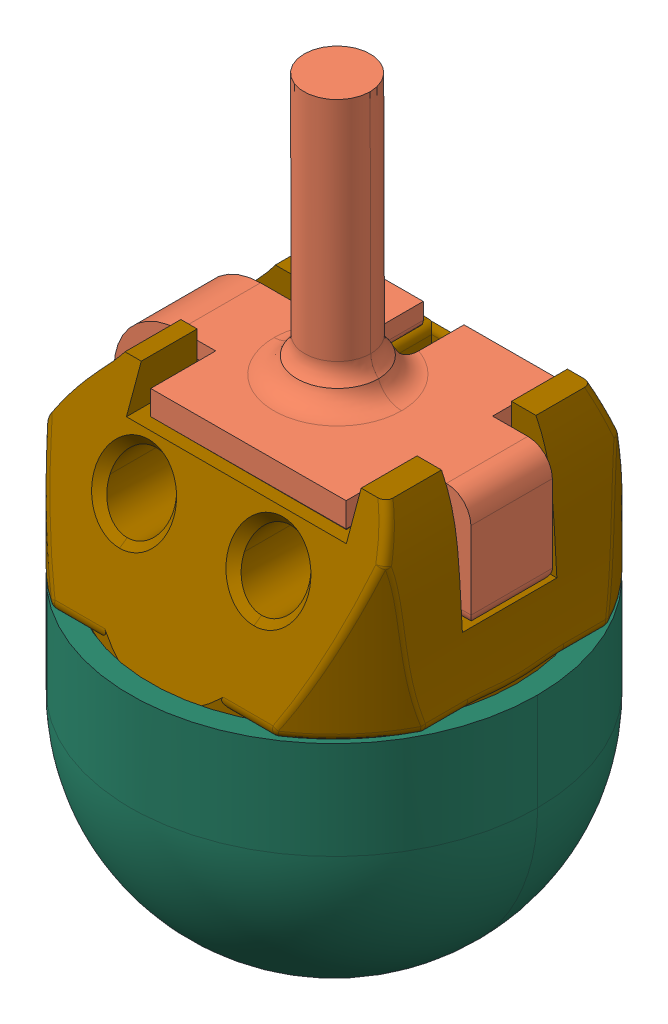
SolidWorks assembly 总装, configuration 默认. Lengths in mm.
Overall size (50 90.92 50).
156 component instances, 58 part files, 0 mates.
Components (placement in the parent):
- 总装(2)^总装-1: 总装(2)^总装 [默认] at origin size (50 90.92 50) (virtual)
  - PCB^总装(2)_总装-1: PCB^总装(2)_总装 [默认] at (-3.2896 -2.1717 0) x (0 0 1) z (0 1 0) size (29.97 29.97 6.79) (virtual)
    - ________.step^PCB_总装(2)_总装-1: ________.step^PCB_总装(2)_总装 [默认] at origin size (29.97 29.97 6.79) (virtual)
      - RES.step^________.step_PCB_总装(2)_总装-1: RES.step^________.step_PCB_总装(2)_总装 [默认] at (9.5064 -1.397 1.6001) x (-1 0 0) z (0 0 1) size (4.88 3 2) (virtual)
        - SW-SMD_L4.0-W3.0-LS4.8.step^RES.step_________.step_PCB_总装(2)_总装-1: SW-SMD_L4.0-W3.0-LS4.8.step^RES.step_________.step_PCB_总装(2)_总装 [默认] at origin size (4.88 3 2) (virtual)
          - COMPOUND.step^SW-SMD_L4.0-W3.0-LS4.8.step_RES.step_________.step_PCB_总装(2)_总装-1: COMPOUND.step^SW-SMD_L4.0-W3.0-LS4.8.step_RES.step_________.step_PCB_总装(2)_总装 [默认] at origin size (4.88 3 2) (virtual)
      - BOOT.step^________.step_PCB_总装(2)_总装-1: BOOT.step^________.step_PCB_总装(2)_总装 [默认] at (-9.435 3.048 1.6001) size (4.88 3 2) (virtual)
        - SW-SMD_L4.0-W3.0-LS4.8.step-1^BOOT.step_________.step_PCB_总装(2)_总装-1: SW-SMD_L4.0-W3.0-LS4.8.step-1^BOOT.step_________.step_PCB_总装(2)_总装 [默认] at origin size (4.88 3 2) (virtual)
          - COMPOUND.step^SW-SMD_L4.0-W3.0-LS4.8.step-1_BOOT.step_________.step_PCB_总装(2)_总装-1: COMPOUND.step^SW-SMD_L4.0-W3.0-LS4.8.step-1_BOOT.step_________.step_PCB_总装(2)_总装 [默认] at origin size (4.88 3 2) (virtual)
      - U1.step^________.step_PCB_总装(2)_总装-1: U1.step^________.step_PCB_总装(2)_总装 [默认] at (0 -10.1196 1.6001) x (0 1 0) z (0 0 1) size (7.02 7.02 0.87) (virtual)
        - LQFN-56_L7.0-W7.0-P0.4-EP.step^U1.step_________.step_PCB_总装(2)_总装-1: LQFN-56_L7.0-W7.0-P0.4-EP.step^U1.step_________.step_PCB_总装(2)_总装 [默认] at origin size (7.02 7.02 0.87) (virtual)
          - SOLID.step^LQFN-56_L7.0-W7.0-P0.4-EP.step_U1.step_________.step_PCB_总装(2)_总装-1: SOLID.step^LQFN-56_L7.0-W7.0-P0.4-EP.step_U1.step_________.step_PCB_总装(2)_总装 [默认] at origin size (7.02 7.02 0.87) (virtual)
      - U4.step^________.step_PCB_总装(2)_总装-1: U4.step^________.step_PCB_总装(2)_总装 [默认] at (-7.62 -11.176 1.6001) x (0.573576 0.819152 0) z (0 0 1) size (0.76 0.76 0.76) (virtual)
        - USON-8_L3.0-W2.0-P0.50-BL-EP.step^U4.step_________.step_PCB_总装(2)_总装-1: USON-8_L3.0-W2.0-P0.50-BL-EP.step^U4.step_________.step_PCB_总装(2)_总装 [默认] at origin size (0.76 0.76 0.76) (virtual)
          - SOLID-0.step^USON-8_L3.0-W2.0-P0.50-BL-EP.step_U4.step_________.step_PCB_总装(2)_总装-1: SOLID-0.step^USON-8_L3.0-W2.0-P0.50-BL-EP.step_U4.step_________.step_PCB_总装(2)_总装 [默认] at origin size (0.76 0.76 0.76) (virtual)
      - R9.step^________.step_PCB_总装(2)_总装-1: R9.step^________.step_PCB_总装(2)_总装 [默认] at (-6.223 -4.953 1.6001) x (0 1 0) z (0 0 1) size (1.62 0.81 0.45) (virtual)
        - R0603.step^R9.step_________.step_PCB_总装(2)_总装-1: R0603.step^R9.step_________.step_PCB_总装(2)_总装 [默认] at origin size (1.62 0.81 0.45) (virtual)
          - COMPOUND-1.step^R0603.step_R9.step_________.step_PCB_总装(2)_总装-1: COMPOUND-1.step^R0603.step_R9.step_________.step_PCB_总装(2)_总装 [默认] at origin size (1.62 0.81 0.45) (virtual)
      - R17.step^________.step_PCB_总装(2)_总装-1: R17.step^________.step_PCB_总装(2)_总装 [默认] at (10.414 -5.842 1.6001) x (-1 0 0) z (0 0 1) size (1.62 0.81 0.45) (virtual)
        - R0603.step-1^R17.step_________.step_PCB_总装(2)_总装-1: R0603.step-1^R17.step_________.step_PCB_总装(2)_总装 [默认] at origin size (1.62 0.81 0.45) (virtual)
          - COMPOUND-1.step^R0603.step-1_R17.step_________.step_PCB_总装(2)_总装-1: COMPOUND-1.step^R0603.step-1_R17.step_________.step_PCB_总装(2)_总装 [默认] at origin size (1.62 0.81 0.45) (virtual)
      - R18.step^________.step_PCB_总装(2)_总装-1: R18.step^________.step_PCB_总装(2)_总装 [默认] at (-4.318 -11.176 0) x (0 1 0) z (0 0 -1) size (1.62 0.81 0.45) (virtual)
        - R0603.step-2^R18.step_________.step_PCB_总装(2)_总装-1: R0603.step-2^R18.step_________.step_PCB_总装(2)_总装 [默认] at origin size (1.62 0.81 0.45) (virtual)
          - COMPOUND-1.step^R0603.step-2_R18.step_________.step_PCB_总装(2)_总装-1: COMPOUND-1.step^R0603.step-2_R18.step_________.step_PCB_总装(2)_总装 [默认] at origin size (1.62 0.81 0.45) (virtual)
      - R19.step^________.step_PCB_总装(2)_总装-1: R19.step^________.step_PCB_总装(2)_总装 [默认] at (6.731 -7.366 1.6001) size (1.62 0.81 0.45) (virtual)
        - R0603.step-3^R19.step_________.step_PCB_总装(2)_总装-1: R0603.step-3^R19.step_________.step_PCB_总装(2)_总装 [默认] at origin size (1.62 0.81 0.45) (virtual)
          - COMPOUND-1.step^R0603.step-3_R19.step_________.step_PCB_总装(2)_总装-1: COMPOUND-1.step^R0603.step-3_R19.step_________.step_PCB_总装(2)_总装 [默认] at origin size (1.62 0.81 0.45) (virtual)
      - R22.step^________.step_PCB_总装(2)_总装-1: R22.step^________.step_PCB_总装(2)_总装 [默认] at (7.2184 -5.842 1.6001) size (1.62 0.81 0.45) (virtual)
        - R0603.step-4^R22.step_________.step_PCB_总装(2)_总装-1: R0603.step-4^R22.step_________.step_PCB_总装(2)_总装 [默认] at origin size (1.62 0.81 0.45) (virtual)
          - COMPOUND-1.step^R0603.step-4_R22.step_________.step_PCB_总装(2)_总装-1: COMPOUND-1.step^R0603.step-4_R22.step_________.step_PCB_总装(2)_总装 [默认] at origin size (1.62 0.81 0.45) (virtual)
      - R23.step^________.step_PCB_总装(2)_总装-1: R23.step^________.step_PCB_总装(2)_总装 [默认] at (7.2184 -4.318 1.6001) size (1.62 0.81 0.45) (virtual)
        - R0603.step-5^R23.step_________.step_PCB_总装(2)_总装-1: R0603.step-5^R23.step_________.step_PCB_总装(2)_总装 [默认] at origin size (1.62 0.81 0.45) (virtual)
          - COMPOUND-1.step^R0603.step-5_R23.step_________.step_PCB_总装(2)_总装-1: COMPOUND-1.step^R0603.step-5_R23.step_________.step_PCB_总装(2)_总装 [默认] at origin size (1.62 0.81 0.45) (virtual)
      - R8.step^________.step_PCB_总装(2)_总装-1: R8.step^________.step_PCB_总装(2)_总装 [默认] at (-7.62 -4.953 1.6001) x (0 1 0) z (0 0 1) size (1.62 0.81 0.45) (virtual)
        - R0603.step-6^R8.step_________.step_PCB_总装(2)_总装-1: R0603.step-6^R8.step_________.step_PCB_总装(2)_总装 [默认] at origin size (1.62 0.81 0.45) (virtual)
          - COMPOUND-1.step^R0603.step-6_R8.step_________.step_PCB_总装(2)_总装-1: COMPOUND-1.step^R0603.step-6_R8.step_________.step_PCB_总装(2)_总装 [默认] at origin size (1.62 0.81 0.45) (virtual)
      - X1.step^________.step_PCB_总装(2)_总装-1: X1.step^________.step_PCB_总装(2)_总装 [默认] at (7.0967 -9.906 1.6001) x (0 1 0) z (0 0 1) size (3.2 2.5 0.81) (virtual)
        - OSC-SMD_4P-L3.2-W2.5-BL.step^X1.step_________.step_PCB_总装(2)_总装-1: OSC-SMD_4P-L3.2-W2.5-BL.step^X1.step_________.step_PCB_总装(2)_总装 [默认] at origin size (3.2 2.5 0.81) (virtual)
          - SOLID-2.step^OSC-SMD_4P-L3.2-W2.5-BL.step_X1.step_________.step_PCB_总装(2)_总装-1: SOLID-2.step^OSC-SMD_4P-L3.2-W2.5-BL.step_X1.step_________.step_PCB_总装(2)_总装 [默认] at origin size (3.2 2.5 0.81) (virtual)
      - LDO1.step^________.step_PCB_总装(2)_总装-1: LDO1.step^________.step_PCB_总装(2)_总装 [默认] at (-9.017 6.454 1.6001) size (2.9 3.01 1.25) (virtual)
        - SOT-23-5_L3.0-W1.7-P0.95-LS2.8-BL.step^LDO1.step_________.step_PCB_总装(2)_总装-1: SOT-23-5_L3.0-W1.7-P0.95-LS2.8-BL.step^LDO1.step_________.step_PCB_总装(2)_总装 [默认] at origin size (2.9 3.01 1.25) (virtual)
          - COMPOUND-3.step^SOT-23-5_L3.0-W1.7-P0.95-LS2.8-BL.step_LDO1.step_________.step_PCB_总装(2)_总装-1: COMPOUND-3.step^SOT-23-5_L3.0-W1.7-P0.95-LS2.8-BL.step_LDO1.step_________.step_PCB_总装(2)_总装 [默认] at origin size (2.9 3.01 1.25) (virtual)
      - C4.step^________.step_PCB_总装(2)_总装-1: C4.step^________.step_PCB_总装(2)_总装 [默认] at (8.8598 1.8415 1.6001) x (0 1 0) z (0 0 1) size (1.6 0.8 0.8) (virtual)
        - C0603.step^C4.step_________.step_PCB_总装(2)_总装-1: C0603.step^C4.step_________.step_PCB_总装(2)_总装 [默认] at origin size (1.6 0.8 0.8) (virtual)
          - SOLID-4.step^C0603.step_C4.step_________.step_PCB_总装(2)_总装-1: SOLID-4.step^C0603.step_C4.step_________.step_PCB_总装(2)_总装 [默认] at origin size (1.6 0.8 0.8) (virtual)
      - C5.step^________.step_PCB_总装(2)_总装-1: C5.step^________.step_PCB_总装(2)_总装 [默认] at (10.2568 1.8415 1.6001) x (0 1 0) z (0 0 1) size (1.6 0.8 0.8) (virtual)
        - C0603.step-1^C5.step_________.step_PCB_总装(2)_总装-1: C0603.step-1^C5.step_________.step_PCB_总装(2)_总装 [默认] at origin size (1.6 0.8 0.8) (virtual)
          - SOLID-4.step^C0603.step-1_C5.step_________.step_PCB_总装(2)_总装-1: SOLID-4.step^C0603.step-1_C5.step_________.step_PCB_总装(2)_总装 [默认] at origin size (1.6 0.8 0.8) (virtual)
      - C6.step^________.step_PCB_总装(2)_总装-1: C6.step^________.step_PCB_总装(2)_总装 [默认] at (11.6538 1.8415 1.6001) x (0 1 0) z (0 0 1) size (1.6 0.8 0.8) (virtual)
        - C0603.step-2^C6.step_________.step_PCB_总装(2)_总装-1: C0603.step-2^C6.step_________.step_PCB_总装(2)_总装 [默认] at origin size (1.6 0.8 0.8) (virtual)
          - SOLID-4.step^C0603.step-2_C6.step_________.step_PCB_总装(2)_总装-1: SOLID-4.step^C0603.step-2_C6.step_________.step_PCB_总装(2)_总装 [默认] at origin size (1.6 0.8 0.8) (virtual)
      - C8.step^________.step_PCB_总装(2)_总装-1: C8.step^________.step_PCB_总装(2)_总装 [默认] at (-12.827 -4.191 1.6001) x (0.642788 0.766044 0) z (0 0 1) size (1.6 0.8 0.8) (virtual)
        - C0603.step-3^C8.step_________.step_PCB_总装(2)_总装-1: C0603.step-3^C8.step_________.step_PCB_总装(2)_总装 [默认] at origin size (1.6 0.8 0.8) (virtual)
          - SOLID-4.step^C0603.step-3_C8.step_________.step_PCB_总装(2)_总装-1: SOLID-4.step^C0603.step-3_C8.step_________.step_PCB_总装(2)_总装 [默认] at origin size (1.6 0.8 0.8) (virtual)
      - C9.step^________.step_PCB_总装(2)_总装-1: C9.step^________.step_PCB_总装(2)_总装 [默认] at (-12.065 -5.207 1.6001) x (0.642788 0.766044 0) z (0 0 1) size (1.6 0.8 0.8) (virtual)
        - C0603.step-4^C9.step_________.step_PCB_总装(2)_总装-1: C0603.step-4^C9.step_________.step_PCB_总装(2)_总装 [默认] at origin size (1.6 0.8 0.8) (virtual)
          - SOLID-4.step^C0603.step-4_C9.step_________.step_PCB_总装(2)_总装-1: SOLID-4.step^C0603.step-4_C9.step_________.step_PCB_总装(2)_总装 [默认] at origin size (1.6 0.8 0.8) (virtual)
      - C10.step^________.step_PCB_总装(2)_总装-1: C10.step^________.step_PCB_总装(2)_总装 [默认] at (-11.303 -6.096 1.6001) x (0.642788 0.766044 0) z (0 0 1) size (1.6 0.8 0.8) (virtual)
        - C0603.step-5^C10.step_________.step_PCB_总装(2)_总装-1: C0603.step-5^C10.step_________.step_PCB_总装(2)_总装 [默认] at origin size (1.6 0.8 0.8) (virtual)
          - SOLID-4.step^C0603.step-5_C10.step_________.step_PCB_总装(2)_总装-1: SOLID-4.step^C0603.step-5_C10.step_________.step_PCB_总装(2)_总装 [默认] at origin size (1.6 0.8 0.8) (virtual)
      - C1.step^________.step_PCB_总装(2)_总装-1: C1.step^________.step_PCB_总装(2)_总装 [默认] at (-4.699 -6.2809 1.6001) x (0 1 0) z (0 0 1) size (1.6 0.8 0.8) (virtual)
        - C0603.step-6^C1.step_________.step_PCB_总装(2)_总装-1: C0603.step-6^C1.step_________.step_PCB_总装(2)_总装 [默认] at origin size (1.6 0.8 0.8) (virtual)
          - SOLID-4.step^C0603.step-6_C1.step_________.step_PCB_总装(2)_总装-1: SOLID-4.step^C0603.step-6_C1.step_________.step_PCB_总装(2)_总装 [默认] at origin size (1.6 0.8 0.8) (virtual)
      - C25.step^________.step_PCB_总装(2)_总装-1: C25.step^________.step_PCB_总装(2)_总装 [默认] at (4.445 -11.557 0) x (0 1 0) z (0 0 -1) size (1.6 0.8 0.8) (virtual)
        - C0603.step-7^C25.step_________.step_PCB_总装(2)_总装-1: C0603.step-7^C25.step_________.step_PCB_总装(2)_总装 [默认] at origin size (1.6 0.8 0.8) (virtual)
          - SOLID-4.step^C0603.step-7_C25.step_________.step_PCB_总装(2)_总装-1: SOLID-4.step^C0603.step-7_C25.step_________.step_PCB_总装(2)_总装 [默认] at origin size (1.6 0.8 0.8) (virtual)
      - C26.step^________.step_PCB_总装(2)_总装-1: C26.step^________.step_PCB_总装(2)_总装 [默认] at (5.969 -12.827 1.6001) x (-0.894427 -0.447214 0) z (0 0 1) size (1.6 0.8 0.8) (virtual)
        - C0603.step-8^C26.step_________.step_PCB_总装(2)_总装-1: C0603.step-8^C26.step_________.step_PCB_总装(2)_总装 [默认] at origin size (1.6 0.8 0.8) (virtual)
          - SOLID-4.step^C0603.step-8_C26.step_________.step_PCB_总装(2)_总装-1: SOLID-4.step^C0603.step-8_C26.step_________.step_PCB_总装(2)_总装 [默认] at origin size (1.6 0.8 0.8) (virtual)
      - C27.step^________.step_PCB_总装(2)_总装-1: C27.step^________.step_PCB_总装(2)_总装 [默认] at (9.5091 -8.89 1.6001) x (0 1 0) z (0 0 1) size (1.6 0.8 0.8) (virtual)
        - C0603.step-9^C27.step_________.step_PCB_总装(2)_总装-1: C0603.step-9^C27.step_________.step_PCB_总装(2)_总装 [默认] at origin size (1.6 0.8 0.8) (virtual)
          - SOLID-4.step^C0603.step-9_C27.step_________.step_PCB_总装(2)_总装-1: SOLID-4.step^C0603.step-9_C27.step_________.step_PCB_总装(2)_总装 [默认] at origin size (1.6 0.8 0.8) (virtual)
      - C28.step^________.step_PCB_总装(2)_总装-1: C28.step^________.step_PCB_总装(2)_总装 [默认] at (-6.8472 5.461 1.6001) x (0 -1 0) z (0 0 1) size (1.6 0.8 0.8) (virtual)
        - C0603.step-10^C28.step_________.step_PCB_总装(2)_总装-1: C0603.step-10^C28.step_________.step_PCB_总装(2)_总装 [默认] at origin size (1.6 0.8 0.8) (virtual)
          - SOLID-4.step^C0603.step-10_C28.step_________.step_PCB_总装(2)_总装-1: SOLID-4.step^C0603.step-10_C28.step_________.step_PCB_总装(2)_总装 [默认] at origin size (1.6 0.8 0.8) (virtual)
      - C29.step^________.step_PCB_总装(2)_总装-1: C29.step^________.step_PCB_总装(2)_总装 [默认] at (-5.5988 5.461 1.6001) x (0 -1 0) z (0 0 1) size (1.6 0.8 0.8) (virtual)
        - C0603.step-11^C29.step_________.step_PCB_总装(2)_总装-1: C0603.step-11^C29.step_________.step_PCB_总装(2)_总装 [默认] at origin size (1.6 0.8 0.8) (virtual)
          - SOLID-4.step^C0603.step-11_C29.step_________.step_PCB_总装(2)_总装-1: SOLID-4.step^C0603.step-11_C29.step_________.step_PCB_总装(2)_总装 [默认] at origin size (1.6 0.8 0.8) (virtual)
      - C30.step^________.step_PCB_总装(2)_总装-1: C30.step^________.step_PCB_总装(2)_总装 [默认] at (-11.303 6.6782 1.6001) x (0 1 0) z (0 0 1) size (1.6 0.8 0.8) (virtual)
        - C0603.step-12^C30.step_________.step_PCB_总装(2)_总装-1: C0603.step-12^C30.step_________.step_PCB_总装(2)_总装 [默认] at origin size (1.6 0.8 0.8) (virtual)
          - SOLID-4.step^C0603.step-12_C30.step_________.step_PCB_总装(2)_总装-1: SOLID-4.step^C0603.step-12_C30.step_________.step_PCB_总装(2)_总装 [默认] at origin size (1.6 0.8 0.8) (virtual)
      - C31.step^________.step_PCB_总装(2)_总装-1: C31.step^________.step_PCB_总装(2)_总装 [默认] at (-9.01 8.89 1.6001) x (-1 0 0) z (0 0 1) size (1.6 0.8 0.8) (virtual)
        - C0603.step-13^C31.step_________.step_PCB_总装(2)_总装-1: C0603.step-13^C31.step_________.step_PCB_总装(2)_总装 [默认] at origin size (1.6 0.8 0.8) (virtual)
          - SOLID-4.step^C0603.step-13_C31.step_________.step_PCB_总装(2)_总装-1: SOLID-4.step^C0603.step-13_C31.step_________.step_PCB_总装(2)_总装 [默认] at origin size (1.6 0.8 0.8) (virtual)
      - C32.step^________.step_PCB_总装(2)_总装-1: C32.step^________.step_PCB_总装(2)_总装 [默认] at (-11.176 -7.5791 1.6001) x (-0.642788 -0.766044 0) z (0 0 1) size (1.6 0.8 0.8) (virtual)
        - C0603.step-14^C32.step_________.step_PCB_总装(2)_总装-1: C0603.step-14^C32.step_________.step_PCB_总装(2)_总装 [默认] at origin size (1.6 0.8 0.8) (virtual)
          - SOLID-4.step^C0603.step-14_C32.step_________.step_PCB_总装(2)_总装-1: SOLID-4.step^C0603.step-14_C32.step_________.step_PCB_总装(2)_总装 [默认] at origin size (1.6 0.8 0.8) (virtual)
      - C33.step^________.step_PCB_总装(2)_总装-1: C33.step^________.step_PCB_总装(2)_总装 [默认] at (-10.16 -8.509 1.6001) x (-0.642788 -0.766044 0) z (0 0 1) size (1.6 0.8 0.8) (virtual)
        - C0603.step-15^C33.step_________.step_PCB_总装(2)_总装-1: C0603.step-15^C33.step_________.step_PCB_总装(2)_总装 [默认] at origin size (1.6 0.8 0.8) (virtual)
          - SOLID-4.step^C0603.step-15_C33.step_________.step_PCB_总装(2)_总装-1: SOLID-4.step^C0603.step-15_C33.step_________.step_PCB_总装(2)_总装 [默认] at origin size (1.6 0.8 0.8) (virtual)
      - C34.step^________.step_PCB_总装(2)_总装-1: C34.step^________.step_PCB_总装(2)_总装 [默认] at (-2.7396 -12.065 0) x (0 1 0) z (0 0 -1) size (1.6 0.8 0.8) (virtual)
        - C0603.step-16^C34.step_________.step_PCB_总装(2)_总装-1: C0603.step-16^C34.step_________.step_PCB_总装(2)_总装 [默认] at origin size (1.6 0.8 0.8) (virtual)
          - SOLID-4.step^C0603.step-16_C34.step_________.step_PCB_总装(2)_总装-1: SOLID-4.step^C0603.step-16_C34.step_________.step_PCB_总装(2)_总装 [默认] at origin size (1.6 0.8 0.8) (virtual)
      - C37.step^________.step_PCB_总装(2)_总装-1: C37.step^________.step_PCB_总装(2)_总装 [默认] at (-12.192 -2.667 0) x (-1 0 0) z (0 0 -1) size (1.6 0.8 0.8) (virtual)
        - C0603.step-17^C37.step_________.step_PCB_总装(2)_总装-1: C0603.step-17^C37.step_________.step_PCB_总装(2)_总装 [默认] at origin size (1.6 0.8 0.8) (virtual)
          - SOLID-4.step^C0603.step-17_C37.step_________.step_PCB_总装(2)_总装-1: SOLID-4.step^C0603.step-17_C37.step_________.step_PCB_总装(2)_总装 [默认] at origin size (1.6 0.8 0.8) (virtual)
      - C38.step^________.step_PCB_总装(2)_总装-1: C38.step^________.step_PCB_总装(2)_总装 [默认] at (2.7397 12.065 0) x (0 -1 0) z (0 0 -1) size (1.6 0.8 0.8) (virtual)
        - C0603.step-18^C38.step_________.step_PCB_总装(2)_总装-1: C0603.step-18^C38.step_________.step_PCB_总装(2)_总装 [默认] at origin size (1.6 0.8 0.8) (virtual)
          - SOLID-4.step^C0603.step-18_C38.step_________.step_PCB_总装(2)_总装-1: SOLID-4.step^C0603.step-18_C38.step_________.step_PCB_总装(2)_总装 [默认] at origin size (1.6 0.8 0.8) (virtual)
      - C40.step^________.step_PCB_总装(2)_总装-1: C40.step^________.step_PCB_总装(2)_总装 [默认] at (11.9509 2.667 0) x (1 0 0) z (0 0 -1) size (1.6 0.8 0.8) (virtual)
        - C0603.step-19^C40.step_________.step_PCB_总装(2)_总装-1: C0603.step-19^C40.step_________.step_PCB_总装(2)_总装 [默认] at origin size (1.6 0.8 0.8) (virtual)
          - SOLID-4.step^C0603.step-19_C40.step_________.step_PCB_总装(2)_总装-1: SOLID-4.step^C0603.step-19_C40.step_________.step_PCB_总装(2)_总装 [默认] at origin size (1.6 0.8 0.8) (virtual)
      - C35.step^________.step_PCB_总装(2)_总装-1: C35.step^________.step_PCB_总装(2)_总装 [默认] at (2.7397 -11.938 0) x (0 -1 0) z (0 0 -1) size (1.6 0.8 0.8) (virtual)
        - C0603.step-20^C35.step_________.step_PCB_总装(2)_总装-1: C0603.step-20^C35.step_________.step_PCB_总装(2)_总装 [默认] at origin size (1.6 0.8 0.8) (virtual)
          - SOLID-4.step^C0603.step-20_C35.step_________.step_PCB_总装(2)_总装-1: SOLID-4.step^C0603.step-20_C35.step_________.step_PCB_总装(2)_总装 [默认] at origin size (1.6 0.8 0.8) (virtual)
      - C36.step^________.step_PCB_总装(2)_总装-1: C36.step^________.step_PCB_总装(2)_总装 [默认] at (-12.1921 2.794 0) x (1 0 0) z (0 0 -1) size (1.6 0.8 0.8) (virtual)
        - C0603.step-21^C36.step_________.step_PCB_总装(2)_总装-1: C0603.step-21^C36.step_________.step_PCB_总装(2)_总装 [默认] at origin size (1.6 0.8 0.8) (virtual)
          - SOLID-4.step^C0603.step-21_C36.step_________.step_PCB_总装(2)_总装-1: SOLID-4.step^C0603.step-21_C36.step_________.step_PCB_总装(2)_总装 [默认] at origin size (1.6 0.8 0.8) (virtual)
      - C39.step^________.step_PCB_总装(2)_总装-1: C39.step^________.step_PCB_总装(2)_总装 [默认] at (-2.794 11.973 0) x (0 1 0) z (0 0 -1) size (1.6 0.8 0.8) (virtual)
        - C0603.step-22^C39.step_________.step_PCB_总装(2)_总装-1: C0603.step-22^C39.step_________.step_PCB_总装(2)_总装 [默认] at origin size (1.6 0.8 0.8) (virtual)
          - SOLID-4.step^C0603.step-22_C39.step_________.step_PCB_总装(2)_总装-1: SOLID-4.step^C0603.step-22_C39.step_________.step_PCB_总装(2)_总装 [默认] at origin size (1.6 0.8 0.8) (virtual)
      - C41.step^________.step_PCB_总装(2)_总装-1: C41.step^________.step_PCB_总装(2)_总装 [默认] at (11.9144 -2.667 0) x (-1 0 0) z (0 0 -1) size (1.6 0.8 0.8) (virtual)
        - C0603.step-23^C41.step_________.step_PCB_总装(2)_总装-1: C0603.step-23^C41.step_________.step_PCB_总装(2)_总装 [默认] at origin size (1.6 0.8 0.8) (virtual)
          - SOLID-4.step^C0603.step-23_C41.step_________.step_PCB_总装(2)_总装-1: SOLID-4.step^C0603.step-23_C41.step_________.step_PCB_总装(2)_总装 [默认] at origin size (1.6 0.8 0.8) (virtual)
      - C2.step^________.step_PCB_总装(2)_总装-1: C2.step^________.step_PCB_总装(2)_总装 [默认] at (7.4628 1.8415 1.6001) x (0 1 0) z (0 0 1) size (1.6 0.8 0.8) (virtual)
        - C0603.step-24^C2.step_________.step_PCB_总装(2)_总装-1: C0603.step-24^C2.step_________.step_PCB_总装(2)_总装 [默认] at origin size (1.6 0.8 0.8) (virtual)
          - SOLID-4.step^C0603.step-24_C2.step_________.step_PCB_总装(2)_总装-1: SOLID-4.step^C0603.step-24_C2.step_________.step_PCB_总装(2)_总装 [默认] at origin size (1.6 0.8 0.8) (virtual)
      - SENSOR2.step^________.step_PCB_总装(2)_总装-1: SENSOR2.step^________.step_PCB_总装(2)_总装 [默认] at (-12 0 0) x (0 -1 0) z (0 0 -1) size (3.02 3.02 0.93) (virtual)
        - VQFN-16_L3.0-W3.0-P0.50-BL-EP1.7.step^SENSOR2.step_________.step_PCB_总装(2)_总装-1: VQFN-16_L3.0-W3.0-P0.50-BL-EP1.7.step^SENSOR2.step_________.step_PCB_总装(2)_总装 [默认] at origin size (3.02 3.02 0.93) (virtual)
          - SOLID-5.step^VQFN-16_L3.0-W3.0-P0.50-BL-EP1.7.step_SENSOR2.step_________.step_PCB_总装(2)_总装-1: SOLID-5.step^VQFN-16_L3.0-W3.0-P0.50-BL-EP1.7.step_SENSOR2.step_________.step_PCB_总装(2)_总装 [默认] at origin size (3.02 3.02 0.93) (virtual)
      - SENSOR3.step^________.step_PCB_总装(2)_总装-1: SENSOR3.step^________.step_PCB_总装(2)_总装 [默认] at (0 12 0) x (-1 0 0) z (0 0 -1) size (3.02 3.02 0.93) (virtual)
        - VQFN-16_L3.0-W3.0-P0.50-BL-EP1.7.step-1^SENSOR3.step_________.step_PCB_总装(2)_总装-1: VQFN-16_L3.0-W3.0-P0.50-BL-EP1.7.step-1^SENSOR3.step_________.step_PCB_总装(2)_总装 [默认] at origin size (3.02 3.02 0.93) (virtual)
          - SOLID-5.step^VQFN-16_L3.0-W3.0-P0.50-BL-EP1.7.step-1_SENSOR3.step_________.step_PCB_总装(2)_总装-1: SOLID-5.step^VQFN-16_L3.0-W3.0-P0.50-BL-EP1.7.step-1_SENSOR3.step_________.step_PCB_总装(2)_总装 [默认] at origin size (3.02 3.02 0.93) (virtual)
      - SENSOR4.step^________.step_PCB_总装(2)_总装-1: SENSOR4.step^________.step_PCB_总装(2)_总装 [默认] at (12 0.0001 0) x (0 1 0) z (0 0 -1) size (3.02 3.02 0.93) (virtual)
        - VQFN-16_L3.0-W3.0-P0.50-BL-EP1.7.step-2^SENSOR4.step_________.step_PCB_总装(2)_总装-1: VQFN-16_L3.0-W3.0-P0.50-BL-EP1.7.step-2^SENSOR4.step_________.step_PCB_总装(2)_总装 [默认] at origin size (3.02 3.02 0.93) (virtual)
          - SOLID-5.step^VQFN-16_L3.0-W3.0-P0.50-BL-EP1.7.step-2_SENSOR4.step_________.step_PCB_总装(2)_总装-1: SOLID-5.step^VQFN-16_L3.0-W3.0-P0.50-BL-EP1.7.step-2_SENSOR4.step_________.step_PCB_总装(2)_总装 [默认] at origin size (3.02 3.02 0.93) (virtual)
      - SENSOR1.step^________.step_PCB_总装(2)_总装-1: SENSOR1.step^________.step_PCB_总装(2)_总装 [默认] at (-0.0001 -12 0) x (1 0 0) z (0 0 -1) size (3.02 3.02 0.93) (virtual)
        - VQFN-16_L3.0-W3.0-P0.50-BL-EP1.7.step-3^SENSOR1.step_________.step_PCB_总装(2)_总装-1: VQFN-16_L3.0-W3.0-P0.50-BL-EP1.7.step-3^SENSOR1.step_________.step_PCB_总装(2)_总装 [默认] at origin size (3.02 3.02 0.93) (virtual)
          - SOLID-5.step^VQFN-16_L3.0-W3.0-P0.50-BL-EP1.7.step-3_SENSOR1.step_________.step_PCB_总装(2)_总装-1: SOLID-5.step^VQFN-16_L3.0-W3.0-P0.50-BL-EP1.7.step-3_SENSOR1.step_________.step_PCB_总装(2)_总装 [默认] at origin size (3.02 3.02 0.93) (virtual)
      - USB2.0.step^________.step_PCB_总装(2)_总装-1: USB2.0.step^________.step_PCB_总装(2)_总装 [默认] at (-9.779 -0.381 1.6001) x (-1 0 0) z (0 0 1) size (7 3.61 4.26) (virtual)
        - CONN-SMD-5P-P1.00_BM05B-SRSS-TB-LF-SN.step^USB2.0.step_________.step_PCB_总装(2)_总装-1: CONN-SMD-5P-P1.00_BM05B-SRSS-TB-LF-SN.step^USB2.0.step_________.step_PCB_总装(2)_总装 [默认] at origin size (7 3.61 4.26) (virtual)
          - COMPOUND-6.step^CONN-SMD-5P-P1.00_BM05B-SRSS-TB-LF-SN.step_USB2.0.step_________.step_PCB_总装(2)_总装-1: COMPOUND-6.step^CONN-SMD-5P-P1.00_BM05B-SRSS-TB-LF-SN.step_USB2.0.step_________.step_PCB_总装(2)_总装 [默认] at origin size (7 3.61 4.26) (virtual)
      - COMPOUND-7.step^________.step_PCB_总装(2)_总装-1: COMPOUND-7.step^________.step_PCB_总装(2)_总装 [默认] at origin size (29.97 29.97 1.6) (virtual)
  - 连接外壳Connect shell^总装(2)_总装-1: 连接外壳Connect shell^总装(2)_总装 [默认] at (-28.2896 -11.0717 -25) size (46.86 34.3 46.18) (virtual)
  - 受压块Compressed block^总装(2)_总装-1: 受压块Compressed block^总装(2)_总装 [默认] at (-3.2896 -34.0717 0) size (44.98 26.51 44.2) (virtual)
  - 钛金属弹簧Titanium metal spring^总装(2)_总装-1: 钛金属弹簧Titanium metal spring^总装(2)_总装 [默认] at (-3.2896 -3.6717 0) x (0.992349 0 -0.123461) z (0 -1 0) size (16.5 17.35 19) (virtual)
  - 缓冲海绵Buffering sponge^总装(2)_总装-1: 缓冲海绵Buffering sponge^总装(2)_总装 [默认] at (-3.2896 -3.0717 0) x (-0.969488 0 0.245139) z (0 -1 0) size (30 30 5) (virtual)
  - 5-10-0.5垫片Gasket^总装(2)_总装-1: 5-10-0.5垫片Gasket^总装(2)_总装 [默认] at (-3.2896 -0.5717 0) size (10 0.5 10) (virtual)
  - 5-20-1垫片Gasket^总装(2)_总装-1: 5-20-1垫片Gasket^总装(2)_总装 [默认] at (-3.2896 -3.1717 0) size (20 1 20) (virtual)
  - 橡胶外壳Rubber casing^总装(2)_总装-1: 橡胶外壳Rubber casing^总装(2)_总装 [默认] at (-3.2896 -13.0717 0) size (50 37 50) (virtual)
  - 环形磁铁Ring magnet^总装(2)_总装-1: 环形磁铁Ring magnet^总装(2)_总装 [默认] at (-3.2896 -10.5717 0) size (26 2 26) (virtual)
  - 螺丝1Screw^总装(2)_总装-1: 螺丝1Screw^总装(2)_总装 [默认] at (-3.2896 1.8283 0) x (1 0 0) z (0 -1 0) size (9.5 9.5 7.5) (virtual)
  - m3螺丝2Screw^总装(2)_总装-1: m3螺丝2Screw^总装(2)_总装 [默认] at (-3.2896 -1.6383 0) x (1 0 0) z (0 1 0) size (5.8 5.8 7) (virtual)
  - m3螺丝2Screw^总装(2)_总装-2: m3螺丝2Screw^总装(2)_总装 [默认] at (-3.2896 -23.9324 0) x (0.591353 0 0.806413) z (0 -1 0) size (5.8 5.8 7) (virtual)
  - 螺丝1Screw^总装(2)_总装-2: 螺丝1Screw^总装(2)_总装 [默认] at (-3.2896 -27.1717 0) x (1 0 0) z (0 1 0) size (9.5 9.5 7.5) (virtual)
  - 填充块Block^总装(2)_总装-1: 填充块Block^总装(2)_总装 [默认] at (-3.2896 -12.0324 0) x (0.591353 0 0.806413) z (-0.806413 0 0.591353) size (6 3.6 6) (virtual)
  - Block^总装(2)_总装-1: Block^总装(2)_总装 [默认] at (-24.1094 6.7256 -25.2516) x (0.999996 0.002812 0) z (-0.002812 0.999996 0) size (43.83 25.98 46) (virtual)
  - m5螺母Nut^总装(2)_总装-1: m5螺母Nut^总装(2)_总装 [默认] at (-3.2896 -25.3717 0) x (0.999997 0 -0.002251) z (0 1 0) size (8 9.24 2.7) (virtual)
  - 扎带Ribbon^总装(2)_总装-1: 扎带Ribbon^总装(2)_总装 [默认] at (-3.2896 -17.0717 13.9) x (0 0 1) z (-1 0 0) size (10.8 7.8 1.8) (virtual)
  - 扎带Ribbon^总装(2)_总装-2: 扎带Ribbon^总装(2)_总装 [默认] at (-19.4823 -17.0717 16.1927) x (0.707107 0 -0.707107) z (0.707107 0 0.707107) size (10.8 7.8 1.8) (virtual)
  - 扎带Ribbon^总装(2)_总装-3: 扎带Ribbon^总装(2)_总装 [默认] at (-26.1896 -17.0717 0) x (1 0 0) z (0 0 1) size (10.8 7.8 1.8) (virtual)
  - 扎带Ribbon^总装(2)_总装-4: 扎带Ribbon^总装(2)_总装 [默认] at (6.5392 -17.0717 9.8288) x (0.707107 0 0.707107) z (-0.707107 0 0.707107) size (10.8 7.8 1.8) (virtual)
  - 扎带Ribbon^总装(2)_总装-5: 扎带Ribbon^总装(2)_总装 [默认] at (10.6104 -17.0717 0) x (1 0 0) z (0 0 1) size (10.8 7.8 1.8) (virtual)
  - 扎带Ribbon^总装(2)_总装-6: 扎带Ribbon^总装(2)_总装 [默认] at (-3.2896 -17.0717 -22.9) x (0 0 1) z (-1 0 0) size (10.8 7.8 1.8) (virtual)
  - 扎带Ribbon^总装(2)_总装-7: 扎带Ribbon^总装(2)_总装 [默认] at (6.5392 -17.0717 -9.8288) x (0.707107 0 -0.707107) z (0.707107 0 0.707107) size (10.8 7.8 1.8) (virtual)
  - 扎带Ribbon^总装(2)_总装-8: 扎带Ribbon^总装(2)_总装 [默认] at (-19.4823 -17.0717 -16.1927) x (0.707107 0 0.707107) z (-0.707107 0 0.707107) size (10.8 7.8 1.8) (virtual)
